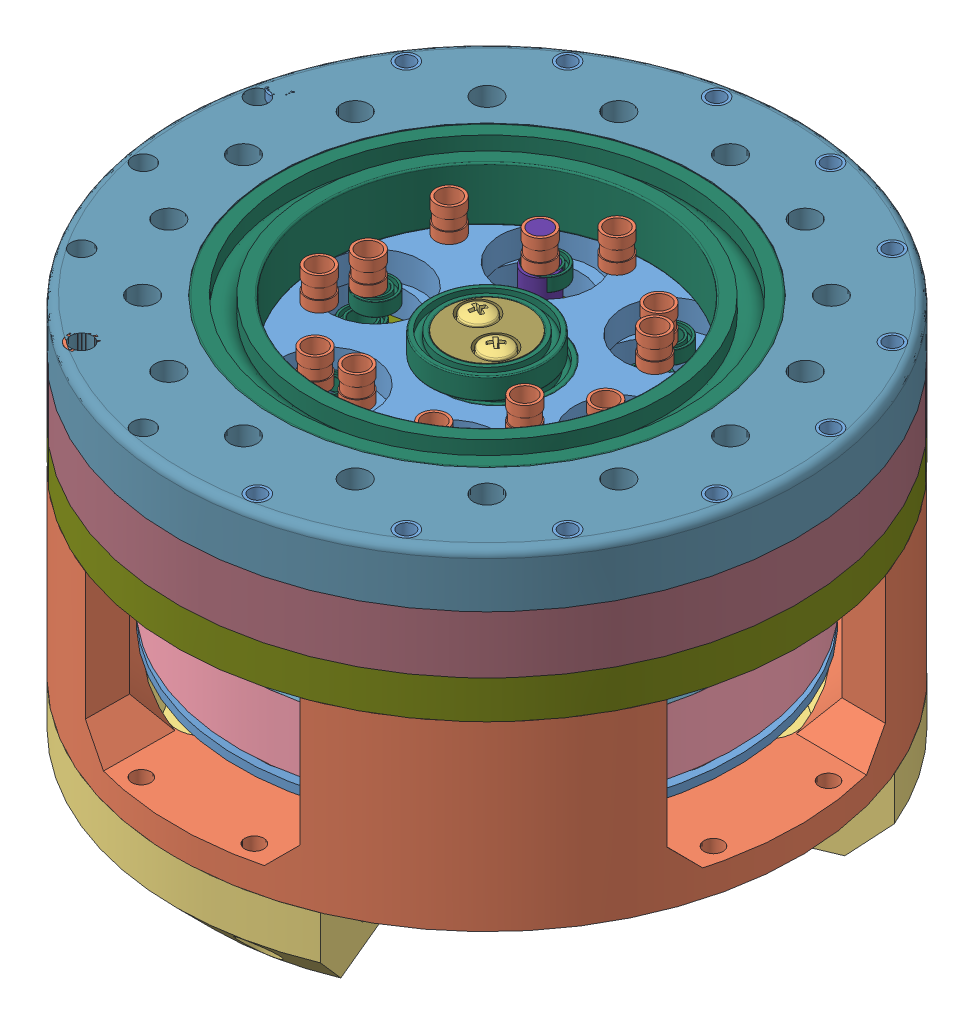
SolidWorks assembly Cycloidal, configuration Default. Lengths in mm.
Overall size (162.63 76.2 162.63).
361 component instances, 94 part files, 194 mates.
Components (placement in the parent):
- motor-X83008S.stp-1: motor-X83008S.stp [Default] at (85.5055 89.7915 110.4458) x (-0.973763 0 -0.227563) z (0 -1 0) size (114.7 114.7 37.62) (hidden)
  - base.stp-1: base.stp [Default] at (42.0794 12.0269 46.7342) size (91.6 91.6 15.61)
  - stator.stp-1: stator.stp [Default] at (42.0794 12.0269 33.1342) x (0.08493 -0.996387 0) z (0 0 1) size (83 83 8)
  - coil.stp-1: coil.stp [Default] at (39.5332 41.8984 37.1342) x (0.996387 0.08493 0) z (-0.08493 0.996387 0) size (4.4 10.2 10.5)
  - coil.stp-2: coil.stp [Default] at (34.3848 41.0025 37.1342) x (0.966502 0.256661 0) z (-0.256661 0.966502 0) size (4.4 10.2 10.5)
  - coil.stp-3: coil.stp [Default] at (29.4701 39.2261 37.1342) x (0.90725 0.420593 0) z (-0.420593 0.90725 0) size (4.4 10.2 10.5)
  - coil.stp-4: coil.stp [Default] at (24.9386 36.6233 37.1342) x (0.820431 0.571745 0) z (-0.571745 0.820431 0) size (4.4 10.2 10.5)
  - coil.stp-5: coil.stp [Default] at (20.9279 33.2732 37.1342) x (0.708685 0.705525 0) z (-0.705525 0.708685 0) size (4.4 10.2 10.5)
  - coil.stp-6: coil.stp [Default] at (17.5599 29.2775 37.1342) x (0.575405 0.817869 0) z (-0.817869 0.575405 0) size (4.4 10.2 10.5)
  - coil.stp-7: coil.stp [Default] at (14.9368 24.7576 37.1342) x (0.424642 0.905361 0) z (-0.905361 0.424642 0) size (4.4 10.2 10.5)
  - coil.stp-8: coil.stp [Default] at (13.1385 19.8509 37.1342) x (0.260976 0.965345 0) z (-0.965345 0.260976 0) size (4.4 10.2 10.5)
  - coil.stp-9: coil.stp [Default] at (12.2196 14.7066 37.1342) x (0.089381 0.995998 0) z (-0.995998 0.089381 0) size (4.4 10.2 10.5)
  - coil.stp-10: coil.stp [Default] at (12.2079 9.4807 37.1342) x (-0.08493 0.996387 0) z (-0.996387 -0.08493 0) size (4.4 10.2 10.5)
  - coil.stp-11: coil.stp [Default] at (13.1039 4.3323 37.1342) x (-0.256661 0.966502 0) z (-0.966502 -0.256661 0) size (4.4 10.2 10.5)
  - coil.stp-12: coil.stp [Default] at (14.8802 -0.5824 37.1342) x (-0.420593 0.90725 0) z (-0.90725 -0.420593 0) size (4.4 10.2 10.5)
  - coil.stp-13: coil.stp [Default] at (17.483 -5.1139 37.1342) x (-0.571745 0.820431 0) z (-0.820431 -0.571745 0) size (4.4 10.2 10.5)
  - coil.stp-14: coil.stp [Default] at (20.8332 -9.1246 37.1342) x (-0.705525 0.708685 0) z (-0.708685 -0.705525 0) size (4.4 10.2 10.5)
  - coil.stp-15: coil.stp [Default] at (24.8289 -12.4926 37.1342) x (-0.817869 0.575405 0) z (-0.575405 -0.817869 0) size (4.4 10.2 10.5)
  - coil.stp-16: coil.stp [Default] at (29.3487 -15.1157 37.1342) x (-0.905361 0.424642 0) z (-0.424642 -0.905361 0) size (4.4 10.2 10.5)
  - coil.stp-17: coil.stp [Default] at (34.2554 -16.914 37.1342) x (-0.965345 0.260976 0) z (-0.260976 -0.965345 0) size (4.4 10.2 10.5)
  - coil.stp-18: coil.stp [Default] at (39.3998 -17.8329 37.1342) x (-0.995998 0.089381 0) z (-0.089381 -0.995998 0) size (4.4 10.2 10.5)
  - coil.stp-19: coil.stp [Default] at (44.6256 -17.8446 37.1342) x (-0.996387 -0.08493 0) z (0.08493 -0.996387 0) size (4.4 10.2 10.5)
  - coil.stp-20: coil.stp [Default] at (49.7741 -16.9486 37.1342) x (-0.966502 -0.256661 0) z (0.256661 -0.966502 0) size (4.4 10.2 10.5)
  - coil.stp-21: coil.stp [Default] at (54.6887 -15.1723 37.1342) x (-0.90725 -0.420593 0) z (0.420593 -0.90725 0) size (4.4 10.2 10.5)
  - coil.stp-22: coil.stp [Default] at (59.2202 -12.5695 37.1342) x (-0.820431 -0.571745 0) z (0.571745 -0.820431 0) size (4.4 10.2 10.5)
  - coil.stp-23: coil.stp [Default] at (63.2309 -9.2193 37.1342) x (-0.708685 -0.705525 0) z (0.705525 -0.708685 0) size (4.4 10.2 10.5)
  - coil.stp-24: coil.stp [Default] at (66.599 -5.2236 37.1342) x (-0.575405 -0.817869 0) z (0.817869 -0.575405 0) size (4.4 10.2 10.5)
  - coil.stp-25: coil.stp [Default] at (69.222 -0.7038 37.1342) x (-0.424642 -0.905361 0) z (0.905361 -0.424642 0) size (4.4 10.2 10.5)
  - coil.stp-26: coil.stp [Default] at (71.0203 4.2029 37.1342) x (-0.260976 -0.965345 0) z (0.965345 -0.260976 0) size (4.4 10.2 10.5)
  - coil.stp-27: coil.stp [Default] at (71.9392 9.3473 37.1342) x (-0.089381 -0.995998 0) z (0.995998 -0.089381 0) size (4.4 10.2 10.5)
  - coil.stp-28: coil.stp [Default] at (71.9509 14.5731 37.1342) x (0.08493 -0.996387 0) z (0.996387 0.08493 0) size (4.4 10.2 10.5)
  - coil.stp-29: coil.stp [Default] at (71.055 19.7216 37.1342) x (0.256661 -0.966502 0) z (0.966502 0.256661 0) size (4.4 10.2 10.5)
  - coil.stp-30: coil.stp [Default] at (69.2786 24.6362 37.1342) x (0.420593 -0.90725 0) z (0.90725 0.420593 0) size (4.4 10.2 10.5)
  - coil.stp-31: coil.stp [Default] at (66.6758 29.1677 37.1342) x (0.571745 -0.820431 0) z (0.820431 0.571745 0) size (4.4 10.2 10.5)
  - coil.stp-32: coil.stp [Default] at (63.3257 33.1785 37.1342) x (0.705525 -0.708685 0) z (0.708685 0.705525 0) size (4.4 10.2 10.5)
  - coil.stp-33: coil.stp [Default] at (59.33 36.5465 37.1342) x (0.817869 -0.575405 0) z (0.575405 0.817869 0) size (4.4 10.2 10.5)
  - coil.stp-34: coil.stp [Default] at (54.8101 39.1695 37.1342) x (0.905361 -0.424642 0) z (0.424642 0.905361 0) size (4.4 10.2 10.5)
  - coil.stp-35: coil.stp [Default] at (49.9034 40.9678 37.1342) x (0.965345 -0.260976 0) z (0.260976 0.965345 0) size (4.4 10.2 10.5)
  - coil.stp-36: coil.stp [Default] at (44.759 41.8868 37.1342) x (0.995998 -0.089381 0) z (0.089381 0.995998 0) size (4.4 10.2 10.5)
  - rotor.stp-1: rotor.stp [Default] at (42.0794 12.0269 42.1342) x (-0.293442 0.955977 0) z (0 0 -1) size (91.8 91.8 12)
  - outrunner.stp-1: outrunner.stp [Default] at (42.0794 12.0269 30.1342) x (-0.254711 0.967017 0) z (-0.967017 -0.254711 0) size (91.8 17.01 91.8)
  - screw-mount.stp-1: screw-mount.stp [Default] at (38.1314 27.0157 27.1342) x (1 0 0) z (0 0 -1) size (7 7 6.5)
  - screw-mount.stp-2: screw-mount.stp [Default] at (27.0906 8.0789 27.1342) x (1 0 0) z (0 0 -1) size (7 7 6.5)
  - screw-mount.stp-3: screw-mount.stp [Default] at (57.0682 15.9749 27.1342) x (1 0 0) z (0 0 -1) size (7 7 6.5)
  - screw-mount.stp-4: screw-mount.stp [Default] at (46.0274 -2.9618 27.1342) x (1 0 0) z (0 0 -1) size (7 7 6.5)
  - 6702ZZ-bearing-15x21x4.stp-1: 6702ZZ-bearing-15x21x4.stp [Default] at (42.0794 12.0269 43.7342) x (1 0 0) z (0 -1 0) size (21 4 21)
  - 6702ZZ-bearing-15x21x4.stp-2: 6702ZZ-bearing-15x21x4.stp [Default] at (42.0794 12.0269 35.1342) x (1 0 0) z (0 1 0) size (21 4 21)
  - shaft.stp-1: shaft.stp [Default] at (42.0794 12.0269 20.1342) size (16 16 31.6)
  - fix-screw.stp-1: fix-screw.stp [Default] at (42.0794 12.0269 51.7342) x (1 0 0) z (0 0 -1) size (19.67 18.96 12.02)
- Base_Plate-1: Base_Plate [Default] at (47.267 69.6573 89.1587) x (0.883683 0 0.468086) z (-0.468086 0 0.883683) size (40 7 40)
- Eccentric_Shaft-1: Eccentric_Shaft [Default] at (31.2439 70.3165 89.3059) x (0.468086 0 -0.883683) z (0.883683 0 0.468086) size (20 15 17)
  - Eccentric_Shaft_bot-1: Eccentric_Shaft_bot [Default] at (7.6302 6.3409 14.0904) size (17 5 17)
  - Eccentric_Shaft_bot-2: Eccentric_Shaft_bot [Default] at (7.6302 11.3409 14.0904) x (-1 0 0) z (0 0 -1) size (17 5 17)
  - Eccentric_Shaft_top-1: Eccentric_Shaft_top [Default] at (7.6302 16.3409 14.0904) x (-1 0 0) z (0 0 -1) size (17 5 17)
- Ring_Pin_Housing-1: Ring_Pin_Housing [Default] at (47.267 76.6573 89.1587) x (0.707107 0 -0.707107) z (0.707107 0 0.707107) size (115 10.6 115)
- Output_Shaft-1: Output_Shaft [Default] at (47.267 87.2573 89.1587) x (0.538744 0 -0.84247) z (0.84247 0 0.538744) size (60 10 60) (hidden)
- Cover-1: Cover [Default] at (47.267 87.2573 89.1587) x (0.707107 0 -0.707107) z (0.707107 0 0.707107) size (115 10.4 115)
- radial ball bearing_68_iso-39: radial ball bearing_68_iso [ISO 15 RBB - 1860 - 32,SI,NC,32_68] at (47.267 92.2573 89.1587) x (0 1 0) z (0 0 1) size (10 78 78)
- radial ball bearing_68_iso-40: radial ball bearing_68_iso [ISO 15 RBB - 1840 - 32,SI,NC,32_68] at (47.267 72.9573 89.1587) x (0 1 0) z (0.001003 0 0.999999) size (7 52 52)
- Base_plate_2-1: Base_plate_2 [Default] at (47.267 69.6573 89.1587) x (0.707107 0 -0.707107) z (0.707107 0 0.707107) size (115 7 115)
- m13_bearing-31: m13_bearing [Default] at (-10.7414 95.4081 67.0593) x (0.227678 0 0.973736) z (0.973736 0 -0.227678) size (13 16 13)
  - m6-1: m6 [Default] at (8.4921 2.5508 14.8914) size (6 16 6)
  - radial ball bearing_68_iso-1: radial ball bearing_68_iso [ISO 15 RBB - 286 - 10,SI,NC,10_68] at (8.4921 16.0508 14.8914) x (0 1 0) z (0 0 1) size (5 13 13)
  - radial ball bearing_68_iso-2: radial ball bearing_68_iso [ISO 15 RBB - 286 - 10,SI,NC,10_68] at (8.4921 11.0508 14.8914) x (0 1 0) z (0 0 1) size (5 13 13)
- m13_bearing-32: m13_bearing [Default] at (-14.1668 95.4081 84.2801) x (0.227678 0 0.973736) z (0.973736 0 -0.227678) size (13 16 13)
  - m6-1: m6 [Default] at (8.4921 2.5508 14.8914) size (6 16 6)
  - radial ball bearing_68_iso-1: radial ball bearing_68_iso [ISO 15 RBB - 286 - 10,SI,NC,10_68] at (8.4921 16.0508 14.8914) x (0 1 0) z (0 0 1) size (5 13 13)
  - radial ball bearing_68_iso-2: radial ball bearing_68_iso [ISO 15 RBB - 286 - 10,SI,NC,10_68] at (8.4921 11.0508 14.8914) x (0 1 0) z (0 0 1) size (5 13 13)
- m13_bearing-34: m13_bearing [Default] at (13.6125 95.5581 125.8547) x (0.227678 0 0.973736) z (0.973736 0 -0.227678) size (13 16 13)
  - m6-1: m6 [Default] at (8.4921 2.5508 14.8914) size (6 16 6)
  - radial ball bearing_68_iso-1: radial ball bearing_68_iso [ISO 15 RBB - 286 - 10,SI,NC,10_68] at (8.4921 16.0508 14.8914) x (0 1 0) z (0 0 1) size (5 13 13)
  - radial ball bearing_68_iso-2: radial ball bearing_68_iso [ISO 15 RBB - 286 - 10,SI,NC,10_68] at (8.4921 11.0508 14.8914) x (0 1 0) z (0 0 1) size (5 13 13)
- m13_bearing-35: m13_bearing [Default] at (-0.9866 95.4081 116.0999) x (0.227678 0 0.973736) z (0.973736 0 -0.227678) size (13 16 13)
  - m6-1: m6 [Default] at (8.4921 2.5508 14.8914) size (6 16 6)
  - radial ball bearing_68_iso-1: radial ball bearing_68_iso [ISO 15 RBB - 286 - 10,SI,NC,10_68] at (8.4921 16.0508 14.8914) x (0 1 0) z (0 0 1) size (5 13 13)
  - radial ball bearing_68_iso-2: radial ball bearing_68_iso [ISO 15 RBB - 286 - 10,SI,NC,10_68] at (8.4921 11.0508 14.8914) x (0 1 0) z (0 0 1) size (5 13 13)
- m13_bearing-36: m13_bearing [Default] at (-10.7414 95.5581 101.5009) x (0.227678 0 0.973736) z (0.973736 0 -0.227678) size (13 16 13)
  - m6-1: m6 [Default] at (8.4921 2.5508 14.8914) size (6 16 6)
  - radial ball bearing_68_iso-1: radial ball bearing_68_iso [ISO 15 RBB - 286 - 10,SI,NC,10_68] at (8.4921 16.0508 14.8914) x (0 1 0) z (0 0 1) size (5 13 13)
  - radial ball bearing_68_iso-2: radial ball bearing_68_iso [ISO 15 RBB - 286 - 10,SI,NC,10_68] at (8.4921 11.0508 14.8914) x (0 1 0) z (0 0 1) size (5 13 13)
- m13_bearing-1: m13_bearing [Default] at (-0.8801 95.4081 62.5627) x (0.736525 0 0.676411) z (0.676411 0 -0.736525) size (13 16 13)
  - m6-1: m6 [Default] at (8.4921 2.5508 14.8914) size (6 16 6)
  - radial ball bearing_68_iso-1: radial ball bearing_68_iso [ISO 15 RBB - 286 - 10,SI,NC,10_68] at (8.4921 16.0508 14.8914) x (0 1 0) z (0 0 1) size (5 13 13)
  - radial ball bearing_68_iso-2: radial ball bearing_68_iso [ISO 15 RBB - 286 - 10,SI,NC,10_68] at (8.4921 11.0508 14.8914) x (0 1 0) z (0 0 1) size (5 13 13)
- m13_bearing-2: m13_bearing [Default] at (48.6831 95.4081 124.0939) x (0.120271 0 0.992741) z (0.992741 0 -0.120271) size (13 16 13)
  - m6-1: m6 [Default] at (8.4921 2.5508 14.8914) size (6 16 6)
  - radial ball bearing_68_iso-1: radial ball bearing_68_iso [ISO 15 RBB - 286 - 10,SI,NC,10_68] at (8.4921 16.0508 14.8914) x (0 1 0) z (0 0 1) size (5 13 13)
  - radial ball bearing_68_iso-2: radial ball bearing_68_iso [ISO 15 RBB - 286 - 10,SI,NC,10_68] at (8.4921 11.0508 14.8914) x (0 1 0) z (0 0 1) size (5 13 13)
- m13_bearing-3: m13_bearing [Default] at (32.7832 95.4081 34.9886) x (-0.046141 0 0.998935) z (0.998935 0 0.046141) size (13 16 13)
  - m6-1: m6 [Default] at (8.4921 2.5508 14.8914) size (6 16 6)
  - radial ball bearing_68_iso-1: radial ball bearing_68_iso [ISO 15 RBB - 286 - 10,SI,NC,10_68] at (8.4921 16.0508 14.8914) x (0 1 0) z (0 0 1) size (5 13 13)
  - radial ball bearing_68_iso-2: radial ball bearing_68_iso [ISO 15 RBB - 286 - 10,SI,NC,10_68] at (8.4921 11.0508 14.8914) x (0 1 0) z (0 0 1) size (5 13 13)
- m13_bearing-4: m13_bearing [Default] at (77.1902 95.4081 81.0003) x (0.022268 0 0.999752) z (0.999752 0 -0.022268) size (13 16 13)
  - m6-1: m6 [Default] at (8.4921 2.5508 14.8914) size (6 16 6)
  - radial ball bearing_68_iso-1: radial ball bearing_68_iso [ISO 15 RBB - 286 - 10,SI,NC,10_68] at (8.4921 16.0508 14.8914) x (0 1 0) z (0 0 1) size (5 13 13)
  - radial ball bearing_68_iso-2: radial ball bearing_68_iso [ISO 15 RBB - 286 - 10,SI,NC,10_68] at (8.4921 11.0508 14.8914) x (0 1 0) z (0 0 1) size (5 13 13)
- m13_bearing-5: m13_bearing [Default] at (73.474 95.4081 98.7828) x (0.059133 0 0.99825) z (0.99825 0 -0.059133) size (13 16 13)
  - m6-1: m6 [Default] at (8.4921 2.5508 14.8914) size (6 16 6)
  - radial ball bearing_68_iso-1: radial ball bearing_68_iso [ISO 15 RBB - 286 - 10,SI,NC,10_68] at (8.4921 16.0508 14.8914) x (0 1 0) z (0 0 1) size (5 13 13)
  - radial ball bearing_68_iso-2: radial ball bearing_68_iso [ISO 15 RBB - 286 - 10,SI,NC,10_68] at (8.4921 11.0508 14.8914) x (0 1 0) z (0 0 1) size (5 13 13)
- m13_bearing-6: m13_bearing [Default] at (12.9248 95.4081 46.7315) x (0.451561 0 0.89224) z (0.89224 0 -0.451561) size (13 16 13)
  - m6-1: m6 [Default] at (8.4921 2.5508 14.8914) size (6 16 6)
  - radial ball bearing_68_iso-1: radial ball bearing_68_iso [ISO 15 RBB - 286 - 10,SI,NC,10_68] at (8.4921 16.0508 14.8914) x (0 1 0) z (0 0 1) size (5 13 13)
  - radial ball bearing_68_iso-2: radial ball bearing_68_iso [ISO 15 RBB - 286 - 10,SI,NC,10_68] at (8.4921 11.0508 14.8914) x (0 1 0) z (0 0 1) size (5 13 13)
- m13_bearing-7: m13_bearing [Default] at (56.6452 95.4081 32.3406) x (-0.545813 0 0.837907) z (0.837907 0 0.545813) size (13 16 13)
  - m6-1: m6 [Default] at (8.4921 2.5508 14.8914) size (6 16 6)
  - radial ball bearing_68_iso-1: radial ball bearing_68_iso [ISO 15 RBB - 286 - 10,SI,NC,10_68] at (8.4921 16.0508 14.8914) x (0 1 0) z (0 0 1) size (5 13 13)
  - radial ball bearing_68_iso-2: radial ball bearing_68_iso [ISO 15 RBB - 286 - 10,SI,NC,10_68] at (8.4921 11.0508 14.8914) x (0 1 0) z (0 0 1) size (5 13 13)
- m13_bearing-8: m13_bearing [Default] at (63.0373 95.4081 51.3153) x (0.158553 0 0.98735) z (0.98735 0 -0.158553) size (13 16 13)
  - m6-1: m6 [Default] at (8.4921 2.5508 14.8914) size (6 16 6)
  - radial ball bearing_68_iso-1: radial ball bearing_68_iso [ISO 15 RBB - 286 - 10,SI,NC,10_68] at (8.4921 16.0508 14.8914) x (0 1 0) z (0 0 1) size (5 13 13)
  - radial ball bearing_68_iso-2: radial ball bearing_68_iso [ISO 15 RBB - 286 - 10,SI,NC,10_68] at (8.4921 11.0508 14.8914) x (0 1 0) z (0 0 1) size (5 13 13)
- m13_bearing-9: m13_bearing [Default] at (83.8577 95.4081 55.5358) x (-0.687134 0 0.72653) z (0.72653 0 0.687134) size (13 16 13)
  - m6-1: m6 [Default] at (8.4921 2.5508 14.8914) size (6 16 6)
  - radial ball bearing_68_iso-1: radial ball bearing_68_iso [ISO 15 RBB - 286 - 10,SI,NC,10_68] at (8.4921 16.0508 14.8914) x (0 1 0) z (0 0 1) size (5 13 13)
  - radial ball bearing_68_iso-2: radial ball bearing_68_iso [ISO 15 RBB - 286 - 10,SI,NC,10_68] at (8.4921 11.0508 14.8914) x (0 1 0) z (0 0 1) size (5 13 13)
- m13_bearing-11: m13_bearing [Default] at (30.1977 95.4081 135.7424) x (0.57351 0 0.819198) z (0.819198 0 -0.57351) size (13 16 13)
  - m6-1: m6 [Default] at (8.4921 2.5508 14.8914) size (6 16 6)
  - radial ball bearing_68_iso-1: radial ball bearing_68_iso [ISO 15 RBB - 286 - 10,SI,NC,10_68] at (8.4921 16.0508 14.8914) x (0 1 0) z (0 0 1) size (5 13 13)
  - radial ball bearing_68_iso-2: radial ball bearing_68_iso [ISO 15 RBB - 286 - 10,SI,NC,10_68] at (8.4921 11.0508 14.8914) x (0 1 0) z (0 0 1) size (5 13 13)
- m13_bearing-12: m13_bearing [Default] at (62.8861 95.4081 115.3744) x (0.184178 0 0.982893) z (0.982893 0 -0.184178) size (13 16 13)
  - m6-1: m6 [Default] at (8.4921 2.5508 14.8914) size (6 16 6)
  - radial ball bearing_68_iso-1: radial ball bearing_68_iso [ISO 15 RBB - 286 - 10,SI,NC,10_68] at (8.4921 16.0508 14.8914) x (0 1 0) z (0 0 1) size (5 13 13)
  - radial ball bearing_68_iso-2: radial ball bearing_68_iso [ISO 15 RBB - 286 - 10,SI,NC,10_68] at (8.4921 11.0508 14.8914) x (0 1 0) z (0 0 1) size (5 13 13)
- socket button head screw_iso-2: socket button head screw_iso [ISO 7380 - M4 x 12 - 12N] at (47.267 67.4573 134.1587) x (0 1 0) z (-0.724148 0 0.689645) size (14.2 7.6 7.6)
- socket button head screw_iso-3: socket button head screw_iso [ISO 7380 - M4 x 12 - 12N] at (15.4472 67.4573 57.3389) x (0 1 0) z (-0.724148 0 0.689645) size (14.2 7.6 7.6)
- socket button head screw_iso-4: socket button head screw_iso [ISO 7380 - M4 x 12 - 12N] at (30.0462 67.4573 47.5841) x (0 1 0) z (-0.724148 0 0.689645) size (14.2 7.6 7.6)
- socket button head screw_iso-5: socket button head screw_iso [ISO 7380 - M4 x 12 - 12N] at (47.267 67.4573 44.1587) x (0 1 0) z (-0.724148 0 0.689645) size (14.2 7.6 7.6)
- socket button head screw_iso-6: socket button head screw_iso [ISO 7380 - M4 x 12 - 12N] at (64.4877 67.4573 47.5841) x (0 1 0) z (-0.724148 0 0.689645) size (14.2 7.6 7.6)
- socket button head screw_iso-8: socket button head screw_iso [ISO 7380 - M4 x 12 - 12N] at (88.8416 67.4573 71.9379) x (0 1 0) z (-0.724148 0 0.689645) size (14.2 7.6 7.6)
- socket button head screw_iso-9: socket button head screw_iso [ISO 7380 - M4 x 12 - 12N] at (92.267 67.4573 89.1587) x (0 1 0) z (-0.724148 0 0.689645) size (14.2 7.6 7.6)
- socket button head screw_iso-10: socket button head screw_iso [ISO 7380 - M4 x 12 - 12N] at (88.8416 67.4573 106.3794) x (0 1 0) z (-0.724148 0 0.689645) size (14.2 7.6 7.6)
- socket button head screw_iso-11: socket button head screw_iso [ISO 7380 - M4 x 12 - 12N] at (79.0868 67.4573 120.9785) x (0 1 0) z (-0.724148 0 0.689645) size (14.2 7.6 7.6)
- M3x4x4.2_brass_insert-1: M3x4x4.2_brass_insert [Default] at (-4.893 93.2573 75.1824) x (0.984609 0 -0.174769) z (0.174769 0 0.984609) size (4 4 4)
- M3x4x4.2_brass_insert-2: M3x4x4.2_brass_insert [Default] at (2.3676 97.2573 59.1579) x (-0.680278 0 -0.732954) z (-0.732954 0 0.680278) size (4 4 4)
- M3x4x4.2_brass_insert-3: M3x4x4.2_brass_insert [Default] at (17.2662 97.2573 44.2593) x (-0.509546 0 -0.860444) z (-0.860444 0 0.509546) size (4 4 4)
- M3x4x4.2_brass_insert-6: M3x4x4.2_brass_insert [Default] at (77.2678 97.2573 44.2593) x (-0.680278 0 -0.732954) z (-0.732954 0 0.680278) size (4 4 4)
- M3x4x4.2_brass_insert-8: M3x4x4.2_brass_insert [Default] at (100.2294 93.2573 78.6238) x (-0.970393 0 0.241533) z (-0.241533 0 -0.970393) size (4 4 4)
- M3x4x4.2_brass_insert-14: M3x4x4.2_brass_insert [Default] at (36.7321 97.2573 36.1963) x (0.509546 0 0.860444) z (0.860444 0 -0.509546) size (4 4 4)
- M3x4x4.2_brass_insert-15: M3x4x4.2_brass_insert [Default] at (57.8019 93.2573 36.1963) x (0.897191 0 -0.441644) z (0.441644 0 0.897191) size (4 4 4)
- M3x4x4.2_brass_insert-16: M3x4x4.2_brass_insert [Default] at (92.1663 97.2573 59.1579) x (-0.680278 0 -0.732954) z (-0.732954 0 0.680278) size (4 4 4)
- M3x4x4.2_brass_insert-17: M3x4x4.2_brass_insert [Default] at (100.2294 97.2573 99.6935) x (0.680278 0 0.732954) z (0.732954 0 -0.680278) size (4 4 4)
- M3x4x4.2_brass_insert-19: M3x4x4.2_brass_insert [Default] at (92.1663 97.2573 119.1595) x (0.680278 0 0.732954) z (0.732954 0 -0.680278) size (4 4 4)
- M3x4x4.2_brass_insert-20: M3x4x4.2_brass_insert [Default] at (77.2678 97.2573 134.058) x (0.680278 0 0.732954) z (0.732954 0 -0.680278) size (4 4 4)
- M3x4x4.2_brass_insert-21: M3x4x4.2_brass_insert [Default] at (57.8019 97.2573 142.1211) x (0.680278 0 0.732954) z (0.732954 0 -0.680278) size (4 4 4)
- M4x6x5.5_brass_insert-47: M4x6x5.5_brass_insert [Default] at (5.6924 92.8573 71.9379) x (0.474598 0 0.880203) z (0 1 0) size (5 5 6)
- M4x6x5.5_brass_insert-48: M4x6x5.5_brass_insert [Default] at (2.267 92.8573 89.1587) x (0.260051 0 0.965595) z (0 1 0) size (5 5 6)
- M4x6x5.5_brass_insert-49: M4x6x5.5_brass_insert [Default] at (5.6924 87.0073 106.3794) x (-0.745833 0 0.666133) z (0 -1 0) size (5 5 6)
- M4x6x5.5_brass_insert-50: M4x6x5.5_brass_insert [Default] at (15.4472 86.8573 120.9785) x (-0.745833 0 0.666133) z (0 -1 0) size (5 5 6)
- M4x6x5.5_brass_insert-51: M4x6x5.5_brass_insert [Default] at (30.0462 87.0073 130.7332) x (0.260051 0 -0.965595) z (0 -1 0) size (5 5 6)
- M4x6x5.5_brass_insert-1: M4x6x5.5_brass_insert [Default] at (70.2433 86.633 90.2013) x (-0.745833 0 0.666133) z (0 -1 0) size (5 5 6)
- M4x6x5.5_brass_insert-4: M4x6x5.5_brass_insert [Default] at (34.8759 92.633 108.5355) x (0.260051 0 0.965595) z (0 1 0) size (5 5 6)
- M4x6x5.5_brass_insert-5: M4x6x5.5_brass_insert [Default] at (24.2906 92.633 88.1161) x (0.260051 0 0.965595) z (0 1 0) size (5 5 6)
- M4x6x5.5_brass_insert-6: M4x6x5.5_brass_insert [Default] at (36.6817 92.633 68.7393) x (0.252509 0 0.967595) z (0 1 0) size (5 5 6)
- M4x6x5.5_brass_insert-7: M4x6x5.5_brass_insert [Default] at (59.6581 92.633 69.7819) x (0.175665 0 0.98445) z (0 1 0) size (5 5 6)
- M4x6x5.5_brass_insert-8: M4x6x5.5_brass_insert [Default] at (66.6438 97.2573 101.5498) x (0.260051 0 0.965595) z (0 1 0) size (5 5 6)
- M4x6x5.5_brass_insert-9: M4x6x5.5_brass_insert [Default] at (67.6864 97.2573 78.5734) x (0.260051 0 0.965595) z (0 1 0) size (5 5 6)
- M4x6x5.5_brass_insert-10: M4x6x5.5_brass_insert [Default] at (48.3096 97.2573 66.1823) x (0.009651 0 0.999953) z (0 1 0) size (5 5 6)
- M4x6x5.5_brass_insert-11: M4x6x5.5_brass_insert [Default] at (27.8902 97.2573 76.7676) x (0.260051 0 0.965595) z (0 1 0) size (5 5 6)
- M4x6x5.5_brass_insert-13: M4x6x5.5_brass_insert [Default] at (26.8476 97.2573 99.7439) x (0.260051 0 0.965595) z (0 1 0) size (5 5 6)
- M4x6x5.5_brass_insert-14: M4x6x5.5_brass_insert [Default] at (46.2244 97.2573 112.135) x (0.260051 0 0.965595) z (0 1 0) size (5 5 6)
- M4x6x5.5_brass_insert-15: M4x6x5.5_brass_insert [Default] at (57.8522 92.633 109.5781) x (0.151918 0 0.988393) z (0 1 0) size (5 5 6)
- M4x6x5.5_brass_insert-20: M4x6x5.5_brass_insert [Default] at (64.4877 86.8573 130.7332) x (-0.745833 0 0.666133) z (0 -1 0) size (5 5 6)
- M4x6x5.5_brass_insert-21: M4x6x5.5_brass_insert [Default] at (47.267 86.8573 134.1587) x (-0.745833 0 0.666133) z (0 -1 0) size (5 5 6)
- M4x6x5.5_brass_insert-22: M4x6x5.5_brass_insert [Default] at (15.4472 86.8573 57.3389) x (0.623293 0 0.781988) z (0 -1 0) size (5 5 6)
- M4x6x5.5_brass_insert-23: M4x6x5.5_brass_insert [Default] at (30.0462 86.8573 47.5841) x (0.623293 0 0.781988) z (0 -1 0) size (5 5 6)
- M4x6x5.5_brass_insert-24: M4x6x5.5_brass_insert [Default] at (79.0868 86.8573 120.9785) x (0.541965 0 0.840401) z (0 -1 0) size (5 5 6)
- M4x6x5.5_brass_insert-25: M4x6x5.5_brass_insert [Default] at (88.8416 86.8573 106.3794) x (-0.745833 0 0.666133) z (0 -1 0) size (5 5 6)
- M4x6x5.5_brass_insert-26: M4x6x5.5_brass_insert [Default] at (92.267 86.8573 89.1587) x (-0.745833 0 0.666133) z (0 -1 0) size (5 5 6)
- M4x6x5.5_brass_insert-27: M4x6x5.5_brass_insert [Default] at (88.8416 86.8573 71.9379) x (-0.745833 0 0.666133) z (0 -1 0) size (5 5 6)
- M4x6x5.5_brass_insert-28: M4x6x5.5_brass_insert [Default] at (79.0868 92.8573 57.3389) x (0.260051 0 0.965595) z (0 1 0) size (5 5 6)
- M4x6x5.5_brass_insert-29: M4x6x5.5_brass_insert [Default] at (64.4877 86.8573 47.5841) x (-0.142939 0 0.989731) z (0 -1 0) size (5 5 6)
- M4x6x5.5_brass_insert-31: M4x6x5.5_brass_insert [Default] at (47.267 86.8573 44.1587) x (-0.220341 0 0.975423) z (0 -1 0) size (5 5 6)
- M4x6x5.5_brass_insert-45: M4x6x5.5_brass_insert [Default] at (17.2662 97.2573 134.058) x (0.260051 0 0.965595) z (0 1 0) size (5 5 6)
- pan cross head_am-1: pan cross head_am [B18.6.7M - M3 x 0.5 x 20 Type I Cross Recessed PHMS --20N] at (50.8017 92.5573 91.031) x (0 -1 0) z (0.748822 0 0.662771) size (22.37 5.6 5.6)
- pan cross head_am-3: pan cross head_am [B18.6.7M - M3 x 0.5 x 20 Type I Cross Recessed PHMS --20N] at (43.7323 92.5573 87.2863) x (0 -1 0) z (0.940321 0 0.340288) size (22.37 5.6 5.6)
- M3x4x4.2_brass_insert-22: M3x4x4.2_brass_insert [Default] at (50.8017 69.6573 91.031) x (0.984609 0 -0.174769) z (0.174769 0 0.984609) size (4 4 4)
- M3x4x4.2_brass_insert-23: M3x4x4.2_brass_insert [Default] at (43.7323 69.6573 87.2863) x (0.984609 0 -0.174769) z (0.174769 0 0.984609) size (4 4 4)
- pan cross head_am-4: pan cross head_am [B18.6.7M - M3 x 0.5 x 10 Type I Cross Recessed PHMS --10N] at (33.5699 77.5573 81.9033) x (0 -1 0) z (0 0 1) size (12.37 5.6 5.6)
- pan cross head_am-5: pan cross head_am [B18.6.7M - M3 x 0.5 x 10 Type I Cross Recessed PHMS --10N] at (60.9641 77.5573 96.414) x (0 -1 0) z (0 0 1) size (12.37 5.6 5.6)
- pan cross head_am-6: pan cross head_am [B18.6.7M - M3 x 0.5 x 10 Type I Cross Recessed PHMS --10N] at (40.0117 77.5573 102.8558) x (0 -1 0) z (0 0 1) size (12.37 5.6 5.6)
- pan cross head_am-7: pan cross head_am [B18.6.7M - M3 x 0.5 x 10 Type I Cross Recessed PHMS --10N] at (54.5223 77.5573 75.4616) x (0 -1 0) z (0 0 1) size (12.37 5.6 5.6)
- radial ball bearing_68_iso-44: radial ball bearing_68_iso [ISO 15 RBB - 1715 - 26,SI,NC,26_68] at (47.9691 84.6573 87.8331) x (0 1 0) z (-0.714953 0 -0.699173) size (4 21 21)
- radial ball bearing_68_iso-45: radial ball bearing_68_iso [ISO 15 RBB - 1715 - 26,SI,NC,26_68] at (47.267 89.6573 89.1587) x (0 1 0) z (0.999483 0 -0.032163) size (4 21 21)
- radial ball bearing_68_iso-46: radial ball bearing_68_iso [ISO 15 RBB - 1715 - 26,SI,NC,26_68] at (46.5649 79.6573 90.4842) x (0 1 0) z (0 0 1) size (4 21 21)
- socket button head screw_iso-37: socket button head screw_iso [ISO 7380 - M4 x 12 - 12N] at (79.0868 67.4573 57.3389) x (0 1 0) z (-0.709975 0 0.704227) size (14.2 7.6 7.6)
- socket button head screw_iso-38: socket button head screw_iso [ISO 7380 - M4 x 12 - 12N] at (64.4877 67.4573 130.7332) x (0 1 0) z (-0.724148 0 0.689645) size (14.2 7.6 7.6)
- foc-motor-controller.step-1: foc-motor-controller.step [Default] at (47.267 33.6573 89.1587) x (0.700658 0 0.713497) z (0 -1 0) size (57.23 50 8.13)
  - RTA0040B.step-1: RTA0040B.step [Default] at (12.5014 -1.6986 1.595) x (-0.707107 -0.707107 0) z (0 0 1) size (6 6 1)
    - FRAME.step-1: FRAME.step [Default] x (1 0 0) z (0 -1 0) size (6 0.2 6)
      - SOLID.step-1: SOLID.step [Default] at origin size (0.4 0.2 0.22)
      - SOLID-0.step-1: SOLID-0.step [Default] at origin size (0.4 0.2 0.22)
      - SOLID-1.step-1: SOLID-1.step [Default] at origin size (0.4 0.2 0.22)
      - SOLID-2.step-1: SOLID-2.step [Default] at origin size (0.4 0.2 0.22)
      - SOLID-3.step-1: SOLID-3.step [Default] at origin size (0.4 0.2 0.22)
      - SOLID-4.step-1: SOLID-4.step [Default] at origin size (0.4 0.2 0.22)
      - SOLID-5.step-1: SOLID-5.step [Default] at origin size (0.4 0.2 0.22)
      - SOLID-6.step-1: SOLID-6.step [Default] at origin size (0.4 0.2 0.22)
      - SOLID-7.step-1: SOLID-7.step [Default] at origin size (0.4 0.2 0.22)
      - SOLID-8.step-1: SOLID-8.step [Default] at origin size (0.4 0.2 0.22)
      - SOLID-9.step-1: SOLID-9.step [Default] at origin size (0.22 0.2 0.4)
      - SOLID-10.step-1: SOLID-10.step [Default] at origin size (0.22 0.2 0.4)
      - SOLID-11.step-1: SOLID-11.step [Default] at origin size (0.22 0.2 0.4)
      - SOLID-12.step-1: SOLID-12.step [Default] at origin size (0.22 0.2 0.4)
      - SOLID-13.step-1: SOLID-13.step [Default] at origin size (0.22 0.2 0.4)
      - SOLID-14.step-1: SOLID-14.step [Default] at origin size (0.22 0.2 0.4)
      - SOLID-15.step-1: SOLID-15.step [Default] at origin size (0.22 0.2 0.4)
      - SOLID-16.step-1: SOLID-16.step [Default] at origin size (0.22 0.2 0.4)
      - SOLID-17.step-1: SOLID-17.step [Default] at origin size (4.15 0.2 4.15)
      - SOLID-18.step-1: SOLID-18.step [Default] at origin size (0.28 0.1 0.28)
      - SOLID-19.step-1: SOLID-19.step [Default] at origin size (0.28 0.1 0.28)
      - SOLID-20.step-1: SOLID-20.step [Default] at origin size (0.28 0.1 0.28)
      - SOLID-21.step-1: SOLID-21.step [Default] at origin size (0.28 0.1 0.28)
      - SOLID-22.step-1: SOLID-22.step [Default] at origin size (0.4 0.2 0.22)
      - SOLID-23.step-1: SOLID-23.step [Default] at origin size (0.4 0.2 0.22)
      - SOLID-24.step-1: SOLID-24.step [Default] at origin size (0.4 0.2 0.22)
      - SOLID-25.step-1: SOLID-25.step [Default] at origin size (0.4 0.2 0.22)
      - SOLID-26.step-1: SOLID-26.step [Default] at origin size (0.4 0.2 0.22)
      - SOLID-27.step-1: SOLID-27.step [Default] at origin size (0.4 0.2 0.22)
      - SOLID-28.step-1: SOLID-28.step [Default] at origin size (0.4 0.2 0.22)
      - SOLID-29.step-1: SOLID-29.step [Default] at origin size (0.4 0.2 0.22)
      - SOLID-30.step-1: SOLID-30.step [Default] at origin size (0.4 0.2 0.22)
      - SOLID-31.step-1: SOLID-31.step [Default] at origin size (0.4 0.2 0.22)
      - SOLID-32.step-1: SOLID-32.step [Default] at origin size (0.22 0.2 0.4)
      - SOLID-33.step-1: SOLID-33.step [Default] at origin size (0.22 0.2 0.4)
      - SOLID-34.step-1: SOLID-34.step [Default] at origin size (0.22 0.2 0.4)
      - SOLID-35.step-1: SOLID-35.step [Default] at origin size (0.22 0.2 0.4)
      - SOLID-36.step-1: SOLID-36.step [Default] at origin size (0.22 0.2 0.4)
      - SOLID-37.step-1: SOLID-37.step [Default] at origin size (0.22 0.2 0.4)
      - SOLID-38.step-1: SOLID-38.step [Default] at origin size (0.22 0.2 0.4)
      - SOLID-39.step-1: SOLID-39.step [Default] at origin size (0.22 0.2 0.4)
      - SOLID-40.step-1: SOLID-40.step [Default] at origin size (0.22 0.2 0.4)
      - SOLID-41.step-1: SOLID-41.step [Default] at origin size (0.22 0.2 0.4)
      - SOLID-42.step-1: SOLID-42.step [Default] at origin size (0.22 0.2 0.4)
      - SOLID-43.step-1: SOLID-43.step [Default] at origin size (0.22 0.2 0.4)
    - BODY.step-1: BODY.step [Default] at (0 0 0.025) x (1 0 0) z (0 -1 0) size (6 0.97 6)
  - Resonator_SMD_Murata_CSTxExxV-3Pin_3.0x1.1mm.step-1: Resonator_SMD_Murata_CSTxExxV-3Pin_3.0x1.1mm.step [Default] at (1.8 -7 1.595) x (0 1 0) z (0 0 1) size (3.2 1.35 0.9)
  - C_0603_1608Metric.step-1: C_0603_1608Metric.step [Default] at (6.2 -16.8 1.595) x (0 -1 0) z (0 0 1) size (1.6 0.8 0.8)
  - R_0603_1608Metric.step-1: R_0603_1608Metric.step [Default] at (11.8 -7.375 1.595) x (0 1 0) z (0 0 1) size (1.6 0.8 0.45)
  - R_0603_1608Metric.step-2: R_0603_1608Metric.step [Default] at (13.8 -16.8 1.595) x (0 1 0) z (0 0 1) size (1.6 0.8 0.45)
  - R_0603_1608Metric.step-3: R_0603_1608Metric.step [Default] at (18.1 -5.36 1.595) size (1.6 0.8 0.45)
  - C_0603_1608Metric.step-2: C_0603_1608Metric.step [Default] at (2.6 -0.5 1.595) x (0 -1 0) z (0 0 1) size (1.6 0.8 0.8)
  - R_0603_1608Metric.step-4: R_0603_1608Metric.step [Default] at (14.6 -11.3 1.595) x (0 1 0) z (0 0 1) size (1.6 0.8 0.45)
  - L_APV_ANR4020.step-1: L_APV_ANR4020.step [Default] at (22.3 -13.7 1.595) x (0 -1 0) z (0 0 1) size (4.02 4 2)
  - C_0603_1608Metric.step-3: C_0603_1608Metric.step [Default] at (0.3 -12.6 1.595) x (-1 0 0) z (0 0 1) size (1.6 0.8 0.8)
  - C_1206_3216Metric.step-1: C_1206_3216Metric.step [Default] at (15.7 11 1.595) x (0 1 0) z (0 0 1) size (3.2 1.6 1.6)
  - C_0603_1608Metric.step-4: C_0603_1608Metric.step [Default] at (0.3 -9.6 1.595) size (1.6 0.8 0.8)
  - R_0603_1608Metric.step-5: R_0603_1608Metric.step [Default] at (12.3 -16.8 1.595) x (0 1 0) z (0 0 1) size (1.6 0.8 0.45)
  - C_0603_1608Metric.step-5: C_0603_1608Metric.step [Default] at (-0.3 -16.6 1.595) x (0 1 0) z (0 0 1) size (1.6 0.8 0.8)
  - R_0603_1608Metric.step-6: R_0603_1608Metric.step [Default] at (10.9 4.1 1.595) size (1.6 0.8 0.45)
  - C_1206_3216Metric.step-2: C_1206_3216Metric.step [Default] at (6.3 11 1.595) x (0 1 0) z (0 0 1) size (3.2 1.6 1.6)
  - XT30PW_2_2_-M.G.B.step-1: XT30PW_2_2_-M.G.B.step [Default] at (-20.5 9.5 1.595) x (0 -1 0) z (-1 0 0) size (15.5 7.1 12.53)
  - R_0603_1608Metric.step-7: R_0603_1608Metric.step [Default] at (0.3 -11.1 1.595) size (1.6 0.8 0.45)
  - C_0603_1608Metric.step-6: C_0603_1608Metric.step [Default] at (19 -0.4 1.595) x (-0.707107 -0.707107 0) z (0 0 1) size (1.6 0.8 0.8)
  - C_1206_3216Metric.step-3: C_1206_3216Metric.step [Default] at (13.3 11 1.595) x (0 1 0) z (0 0 1) size (3.2 1.6 1.6)
  - R_0603_1608Metric.step-8: R_0603_1608Metric.step [Default] at (10.2 -7.375 1.595) x (0 -1 0) z (0 0 1) size (1.6 0.8 0.45)
  - JST_GH_SM08B-GHS-TB_1x08-1MP_P1.25mm_Horizontal.step-1: JST_GH_SM08B-GHS-TB_1x08-1MP_P1.25mm_Horizontal.step [Default] at (10 -22 1.595) size (13.25 4.95 4.25)
  - C_1206_3216Metric.step-4: C_1206_3216Metric.step [Default] at (-12.3 11 1.595) x (0 1 0) z (0 0 1) size (3.2 1.6 1.6)
  - JST_GH_SM06B-GHS-TB_1x06-1MP_P1.25mm_Horizontal.step-1: JST_GH_SM06B-GHS-TB_1x06-1MP_P1.25mm_Horizontal.step [Default] at (-4.3 -22 1.595) size (10.75 4.95 4.25)
  - C_0603_1608Metric.step-7: C_0603_1608Metric.step [Default] at (7.3 -4.5 1.595) x (-1 0 0) z (0 0 1) size (1.6 0.8 0.8)
  - R_0603_1608Metric.step-9: R_0603_1608Metric.step [Default] at (18.1 -3.86 1.595) x (-1 0 0) z (0 0 1) size (1.6 0.8 0.45)
  - C_1206_3216Metric.step-5: C_1206_3216Metric.step [Default] at (22.6794 -1.2206 1.595) x (0.707107 -0.707107 0) z (0 0 1) size (3.2 1.6 1.6)
  - R_Array_Convex_4x0402.step-1: R_Array_Convex_4x0402.step [Default] at (6.8 -2.5 1.595) size (1 2 0.35)
  - R_0603_1608Metric.step-10: R_0603_1608Metric.step [Default] at (7.7 -16.8 1.595) x (0 -1 0) z (0 0 1) size (1.6 0.8 0.45)
  - C_1206_3216Metric.step-6: C_1206_3216Metric.step [Default] at (8.7 11 1.595) x (0 1 0) z (0 0 1) size (3.2 1.6 1.6)
  - C_0603_1608Metric.step-8: C_0603_1608Metric.step [Default] at (16.1 -11.3 1.595) x (0 1 0) z (0 0 1) size (1.6 0.8 0.8)
  - SOT-23-5.step-1: SOT-23-5.step [Default] at (-3.1 -16.6 1.595) x (-1 0 0) z (0 0 1) size (2.8 2.9 1.55)
  - C_0603_1608Metric.step-9: C_0603_1608Metric.step [Default] at (17.8 -13.6 1.595) size (1.6 0.8 0.8)
  - R_0603_1608Metric.step-11: R_0603_1608Metric.step [Default] at (-11.5 -20.3875 1.595) x (0 -1 0) z (0 0 1) size (1.6 0.8 0.45)
  - C_0603_1608Metric.step-10: C_0603_1608Metric.step [Default] at (-12.4 2.3 1.595) x (0 1 0) z (0 0 1) size (1.6 0.8 0.8)
  - C_1206_3216Metric.step-7: C_1206_3216Metric.step [Default] at (18 11 1.595) x (0 1 0) z (0 0 1) size (3.2 1.6 1.6)
  - R_0603_1608Metric.step-12: R_0603_1608Metric.step [Default] at (-10.8105 -14.9971 1.595) x (-1 0 0) z (0 0 1) size (1.6 0.8 0.45)
  - C_0603_1608Metric.step-11: C_0603_1608Metric.step [Default] at (-13.8 -9.4 1.595) x (-1 0 0) z (0 0 1) size (1.6 0.8 0.8)
  - R_0603_1608Metric.step-13: R_0603_1608Metric.step [Default] at (-23.15 -14.5 1.595) x (-1 0 0) z (0 0 1) size (1.6 0.8 0.45)
  - C_0603_1608Metric.step-12: C_0603_1608Metric.step [Default] at (1.1 -0.2 1.595) x (0 1 0) z (0 0 1) size (1.6 0.8 0.8)
  - D_0805_2012Metric.step-1: D_0805_2012Metric.step [Default] at (22.9 -9.6 1.595) x (0 1 0) z (0 0 1) size (2 1.27 0.8)
  - C_0603_1608Metric.step-13: C_0603_1608Metric.step [Default] at (-7.8 3.775 1.595) x (0 -1 0) z (0 0 1) size (1.6 0.8 0.8)
  - R_0603_1608Metric.step-14: R_0603_1608Metric.step [Default] at (-6.4 -12.825 1.595) x (0 1 0) z (0 0 1) size (1.6 0.8 0.45)
  - L_0603_1608Metric.step-1: L_0603_1608Metric.step [Default] at (-10.1 3 1.595) size (1.6 0.8 0.8)
  - C_0603_1608Metric.step-14: C_0603_1608Metric.step [Default] at (17.9 0.7 1.595) x (-0.707107 -0.707107 0) z (0 0 1) size (1.6 0.8 0.8)
  - HVSSOP-10.step-1: HVSSOP-10.step [Default] at (18.6 -9.6 1.595) x (0 -1 0) z (-1 0 0) size (4.9 1.1 3)
  - C_0603_1608Metric.step-15: C_0603_1608Metric.step [Default] at (7.9 4.1 1.595) x (-1 0 0) z (0 0 1) size (1.6 0.8 0.8)
  - C_0603_1608Metric.step-16: C_0603_1608Metric.step [Default] at (21.1 -9.6 1.595) x (0 -1 0) z (0 0 1) size (1.6 0.8 0.8)
  - R_0603_1608Metric.step-15: R_0603_1608Metric.step [Default] at (-10.8105 -11.9971 1.595) x (-1 0 0) z (0 0 1) size (1.6 0.8 0.45)
  - R_0603_1608Metric.step-16: R_0603_1608Metric.step [Default] at (-18.2 -17.4 1.595) size (1.6 0.8 0.45)
  - C_1206_3216Metric.step-8: C_1206_3216Metric.step [Default] at (-3 11 1.595) x (0 1 0) z (0 0 1) size (3.2 1.6 1.6)
  - R_0603_1608Metric.step-17: R_0603_1608Metric.step [Default] at (-16.9 -20.4 1.595) x (0 -1 0) z (0 0 1) size (1.6 0.8 0.45)
  - R_0603_1608Metric.step-18: R_0603_1608Metric.step [Default] at (-13.3 -20.3875 1.595) x (0 -1 0) z (0 0 1) size (1.6 0.8 0.45)
  - R_0603_1608Metric.step-19: R_0603_1608Metric.step [Default] at (-15.1 -20.3875 1.595) x (0 -1 0) z (0 0 1) size (1.6 0.8 0.45)
  - C_0603_1608Metric.step-17: C_0603_1608Metric.step [Default] at (15.5 -14.4 1.595) x (0 -1 0) z (0 0 1) size (1.6 0.8 0.8)
  - LED_0603_1608Metric.step-1: LED_0603_1608Metric.step [Default] at (-11.5 -23.3875 1.595) x (0 1 0) z (0 0 1) size (1.6 0.8 1.1)
  - C_0805_2012Metric.step-1: C_0805_2012Metric.step [Default] at (19.95 -17 1.595) size (2 1.25 1.25)
  - D_SMB.step-1: D_SMB.step [Default] at (-16.5 11.208 1.595) x (0 -1 0) z (0 0 1) size (5.3 3.55 2.15)
  - C_1206_3216Metric.step-9: C_1206_3216Metric.step [Default] at (-5.3 11 1.595) x (0 1 0) z (0 0 1) size (3.2 1.6 1.6)
  - XT30PW_2_2_-M.G.B.step-2: XT30PW_2_2_-M.G.B.step [Default] at (-20.5 -6.5 1.595) x (0 -1 0) z (-1 0 0) size (15.5 7.1 12.53)
  - C_1206_3216Metric.step-10: C_1206_3216Metric.step [Default] at (1.7 11 1.595) x (0 1 0) z (0 0 1) size (3.2 1.6 1.6)
  - C_1206_3216Metric.step-11: C_1206_3216Metric.step [Default] at (11 11 1.595) x (0 1 0) z (0 0 1) size (3.2 1.6 1.6)
  - C_0603_1608Metric.step-18: C_0603_1608Metric.step [Default] at (-6.3 3.775 1.595) x (0 -1 0) z (0 0 1) size (1.6 0.8 0.8)
  - C_0603_1608Metric.step-19: C_0603_1608Metric.step [Default] at (16.8686 1.7314 1.595) x (0.707107 0.707107 0) z (0 0 1) size (1.6 0.8 0.8)
  - C_0603_1608Metric.step-20: C_0603_1608Metric.step [Default] at (-15.0105 -11.1 1.595) size (1.6 0.8 0.8)
  - C_1206_3216Metric.step-12: C_1206_3216Metric.step [Default] at (-7.7 11 1.595) x (0 1 0) z (0 0 1) size (3.2 1.6 1.6)
  - C_0603_1608Metric.step-21: C_0603_1608Metric.step [Default] at (-18.2 -15.8 1.595) size (1.6 0.8 0.8)
  - C_0603_1608Metric.step-22: C_0603_1608Metric.step [Default] at (-2.1 -11.3 1.595) x (0 -1 0) z (0 0 1) size (1.6 0.8 0.8)
  - C_0603_1608Metric.step-23: C_0603_1608Metric.step [Default] at (-10.8105 -13.4971 1.595) size (1.6 0.8 0.8)
  - C_1206_3216Metric.step-13: C_1206_3216Metric.step [Default] at (4 11 1.595) x (0 1 0) z (0 0 1) size (3.2 1.6 1.6)
  - R_0603_1608Metric.step-20: R_0603_1608Metric.step [Default] at (16 -17.8 1.595) x (0 1 0) z (0 0 1) size (1.6 0.8 0.45)
  - Texas_S-PVSON-N8.step-1: Texas_S-PVSON-N8.step [Default] at (-14.4105 -13.7 1.595) x (-1 0 0) z (0 0 1) size (3 2.98 0.92)
  - C_1206_3216Metric.step-14: C_1206_3216Metric.step [Default] at (21 -2.9 1.595) x (0.707107 -0.707107 0) z (0 0 1) size (3.2 1.6 1.6)
  - C_0603_1608Metric.step-24: C_0603_1608Metric.step [Default] at (-5.9 -16.6 1.595) x (0 1 0) z (0 0 1) size (1.6 0.8 0.8)
  - C_0603_1608Metric.step-25: C_0603_1608Metric.step [Default] at (-3.1 -14.1 1.595) size (1.6 0.8 0.8)
  - R_0603_1608Metric.step-21: R_0603_1608Metric.step [Default] at (7.2 -7.375 1.595) x (0 -1 0) z (0 0 1) size (1.6 0.8 0.45)
  - C_1206_3216Metric.step-15: C_1206_3216Metric.step [Default] at (-0.7 11 1.595) x (0 1 0) z (0 0 1) size (3.2 1.6 1.6)
  - LQFP-64_10x10mm_P0.5mm.step-1: LQFP-64_10x10mm_P0.5mm.step [Default] at (-7 -4.5 1.595) x (-1 0 0) z (0 0 1) size (12 12 1.5)
  - C_0805_2012Metric.step-2: C_0805_2012Metric.step [Default] at (23.35 -17 1.595) x (-1 0 0) z (0 0 1) size (2 1.25 1.25)
  - C_0603_1608Metric.step-26: C_0603_1608Metric.step [Default] at (10.8 -16.8 1.595) x (0 -1 0) z (0 0 1) size (1.6 0.8 0.8)
  - R_0603_1608Metric.step-22: R_0603_1608Metric.step [Default] at (17.5 -17.8 1.595) x (0 -1 0) z (0 0 1) size (1.6 0.8 0.45)
  - C_1206_3216Metric.step-16: C_1206_3216Metric.step [Default] at (20.3 11 1.595) x (0 1 0) z (0 0 1) size (3.2 1.6 1.6)
  - R_0603_1608Metric.step-23: R_0603_1608Metric.step [Default] at (9.2 -16.8 1.595) x (0 -1 0) z (0 0 1) size (1.6 0.8 0.45)
  - C_1206_3216Metric.step-17: C_1206_3216Metric.step [Default] at (-10 11 1.595) x (0 1 0) z (0 0 1) size (3.2 1.6 1.6)
  - R_0603_1608Metric.step-24: R_0603_1608Metric.step [Default] at (17.8 -15.2 1.595) size (1.6 0.8 0.45)
  - C_1206_3216Metric.step-18: C_1206_3216Metric.step [Default] at (19.9 2.6 1.595) x (-0.707107 0.707107 0) z (0 0 1) size (3.2 1.6 1.6)
  - C_0603_1608Metric.step-27: C_0603_1608Metric.step [Default] at (13.4 -7.375 1.595) x (0 -1 0) z (0 0 1) size (1.6 0.8 0.8)
  - R_0603_1608Metric.step-25: R_0603_1608Metric.step [Default] at (8.7 -7.375 1.595) x (0 -1 0) z (0 0 1) size (1.6 0.8 0.45)
  - PQFN-8-EP_6x5mm_P1.27mm_Generic.step-1: PQFN-8-EP_6x5mm_P1.27mm_Generic.step [Default] at (4.9 14.4 -0.085) x (0 1 0) z (0 0 -1) size (6.15 5.15 1.09)
  - C_0805_2012Metric.step-3: C_0805_2012Metric.step [Default] at (-3 8.9 -0.085) x (0 1 0) z (0 0 -1) size (2 1.25 1.25)
  - C_0603_1608Metric.step-28: C_0603_1608Metric.step [Default] at (1.5 -4.3 -0.085) x (0 1 0) z (0 0 -1) size (1.6 0.8 0.8)
  - R_2512_6332Metric.step-1: R_2512_6332Metric.step [Default] at (2.1 8.6 -0.085) x (-1 0 0) z (0 0 -1) size (6.3 3.2 0.6)
  - C_0805_2012Metric.step-4: C_0805_2012Metric.step [Default] at (18.8 8.9 -0.085) x (0 1 0) z (0 0 -1) size (2 1.25 1.25)
  - C_0805_2012Metric.step-5: C_0805_2012Metric.step [Default] at (-5.2 8.901 -0.085) x (0 1 0) z (0 0 -1) size (2 1.25 1.25)
  - PQFN-8-EP_6x5mm_P1.27mm_Generic.step-2: PQFN-8-EP_6x5mm_P1.27mm_Generic.step [Default] at (16.9 14.6 -0.085) x (0 -1 0) z (0 0 -1) size (6.15 5.15 1.09)
  - PQFN-8-EP_6x5mm_P1.27mm_Generic.step-3: PQFN-8-EP_6x5mm_P1.27mm_Generic.step [Default] at (-1.1 14.6 -0.085) x (0 -1 0) z (0 0 -1) size (6.15 5.15 1.09)
  - R_0603_1608Metric.step-26: R_0603_1608Metric.step [Default] at (8.2 8.8 -0.085) x (0 1 0) z (0 0 -1) size (1.6 0.8 0.45)
  - R_2512_6332Metric.step-2: R_2512_6332Metric.step [Default] at (-10.3 8.601 -0.085) x (1 0 0) z (0 0 -1) size (6.3 3.2 0.6)
  - TSSOP-16_4.4x5mm_P0.65mm.step-1: TSSOP-16_4.4x5mm_P0.65mm.step [Default] at (0 0 -0.085) x (-1 0 0) z (0 0 -1) size (6.4 5 1.1)
  - C_0603_1608Metric.step-29: C_0603_1608Metric.step [Default] at (0 -4.25 -0.085) x (0 1 0) z (0 0 -1) size (1.6 0.8 0.8)
  - PQFN-8-EP_6x5mm_P1.27mm_Generic.step-4: PQFN-8-EP_6x5mm_P1.27mm_Generic.step [Default] at (10.9 14.4 -0.085) x (0 1 0) z (0 0 -1) size (6.15 5.15 1.09)
  - R_2512_6332Metric.step-3: R_2512_6332Metric.step [Default] at (13.7 8.6 -0.085) x (1 0 0) z (0 0 -1) size (6.3 3.2 0.6)
  - PQFN-8-EP_6x5mm_P1.27mm_Generic.step-5: PQFN-8-EP_6x5mm_P1.27mm_Generic.step [Default] at (-13.1 14.401 -0.085) x (0 1 0) z (0 0 -1) size (6.15 5.15 1.09)
  - C_0603_1608Metric.step-30: C_0603_1608Metric.step [Default] at (-1.5 -4.3 -0.085) x (0 -1 0) z (0 0 -1) size (1.6 0.8 0.8)
  - PQFN-8-EP_6x5mm_P1.27mm_Generic.step-6: PQFN-8-EP_6x5mm_P1.27mm_Generic.step [Default] at (-7.1 14.601 -0.085) x (0 -1 0) z (0 0 -1) size (6.15 5.15 1.09)
  - foc-motor-controller_PCB.step-1: foc-motor-controller_PCB.step [Default] at origin size (50 50 1.51)
